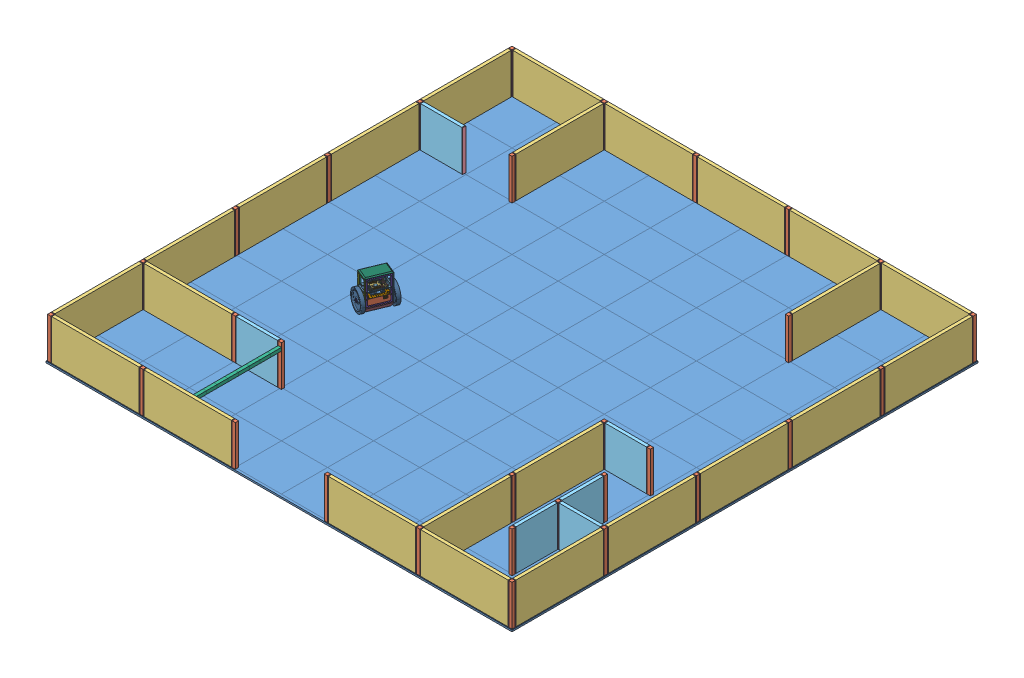
SolidWorks assembly testbed, configuration Default. Lengths in mm.
Overall size (2880 260 2880).
673 component instances, 79 part files, 153 mates.
Components (placement in the parent):
- floor-1: floor [Default] at origin size (2880 10 2880)
- post_250-1: post_250 [Default] at (-2707.5 10 -2707.5) size (20 250 20)
- post_250-2: post_250 [Default] at (-2137.5 10 -2707.5) size (20 250 20)
- post_250-3: post_250 [Default] at (-1567.5 10 -2707.5) size (20 250 20)
- post_250-4: post_250 [Default] at (-997.5 10 -2707.5) size (20 250 20)
- post_250-5: post_250 [Default] at (-427.5 10 -2707.5) size (20 250 20)
- post_250-6: post_250 [Default] at (142.5 10 -2707.5) size (20 250 20)
- post_250-7: post_250 [Default] at (-427.5 10 -2137.5) size (20 250 20)
- post_250-8: post_250 [Default] at (142.5 10 -2137.5) size (20 250 20)
- post_250-9: post_250 [Default] at (-2707.5 10 -2137.5) size (20 250 20)
- post_250-10: post_250 [Default] at (-2707.5 10 -1567.5) size (20 250 20)
- post_250-11: post_250 [Default] at (-2707.5 10 -997.5) size (20 250 20)
- post_250-12: post_250 [Default] at (-2707.5 10 -427.5) size (20 250 20)
- post_250-13: post_250 [Default] at (-2707.5 10 142.5) size (20 250 20)
- post_250-14: post_250 [Default] at (-2137.5 10 142.5) size (20 250 20)
- post_250-15: post_250 [Default] at (-2137.5 10 -427.5) size (20 250 20)
- post_250-16: post_250 [Default] at (-1567.5 10 142.5) size (20 250 20)
- post_250-17: post_250 [Default] at (-997.5 10 142.5) size (20 250 20)
- post_250-18: post_250 [Default] at (-427.5 10 142.5) size (20 250 20)
- post_250-19: post_250 [Default] at (142.5 10 142.5) size (20 250 20)
- post_250-20: post_250 [Default] at (142.5 10 -427.5) size (20 250 20)
- post_250-21: post_250 [Default] at (142.5 10 -997.5) size (20 250 20)
- post_250-22: post_250 [Default] at (142.5 10 -1567.5) size (20 250 20)
- post_250-23: post_250 [Default] at (-2137.5 10 -2137.5) size (20 250 20)
- post_250-24: post_250 [Default] at (-142.5 10 -142.5) size (20 250 20)
- post_250-25: post_250 [Default] at (-427.5 10 -427.5) size (20 250 20)
- post_250-26: post_250 [Default] at (-427.5 10 -997.5) size (20 250 20)
- post_250-27: post_250 [Default] at (-142.5 10 -427.5) size (20 250 20)
- post_250-28: post_250 [Default] at (-142.5 10 -712.5) size (20 250 20)
- post_250-29: post_250 [Default] at (-142.5 10 -997.5) size (20 250 20)
- wallelement_2-cell-1: wallelement_2-cell [Default] at (-712.5 135 132.5) size (550 250 20)
  - wall_2-cell-1: wall_2-cell [Default] at origin size (540 250 20)
  - wall_profile_hook_250-1: wall_profile_hook_250 [Default] at (275 0 10) x (0 0 1) z (-1 0 0) size (20 250 5)
  - wall_profile_hook_250-2: wall_profile_hook_250 [Default] at (-275 0 10) x (0 0 -1) z (1 0 0) size (20 250 5)
- wallelement_2-cell-2: wallelement_2-cell [Default] at (-142.5 135 132.5) size (550 250 20)
  - wall_2-cell-1: wall_2-cell [Default] at origin size (540 250 20)
  - wall_profile_hook_250-1: wall_profile_hook_250 [Default] at (275 0 10) x (0 0 1) z (-1 0 0) size (20 250 5)
  - wall_profile_hook_250-2: wall_profile_hook_250 [Default] at (-275 0 10) x (0 0 -1) z (1 0 0) size (20 250 5)
- wallelement_2-cell-3: wallelement_2-cell [Default] at (132.5 135 -142.5) x (0 0 -1) z (1 0 0) size (550 250 20)
  - wall_2-cell-1: wall_2-cell [Default] at origin size (540 250 20)
  - wall_profile_hook_250-1: wall_profile_hook_250 [Default] at (275 0 10) x (0 0 1) z (-1 0 0) size (20 250 5)
  - wall_profile_hook_250-2: wall_profile_hook_250 [Default] at (-275 0 10) x (0 0 -1) z (1 0 0) size (20 250 5)
- wallelement_2-cell-4: wallelement_2-cell [Default] at (132.5 135 -712.5) x (0 0 -1) z (1 0 0) size (550 250 20)
  - wall_2-cell-1: wall_2-cell [Default] at origin size (540 250 20)
  - wall_profile_hook_250-1: wall_profile_hook_250 [Default] at (275 0 10) x (0 0 1) z (-1 0 0) size (20 250 5)
  - wall_profile_hook_250-2: wall_profile_hook_250 [Default] at (-275 0 10) x (0 0 -1) z (1 0 0) size (20 250 5)
- wallelement_2-cell-5: wallelement_2-cell [Default] at (132.5 135 -1282.5) x (0 0 -1) z (1 0 0) size (550 250 20)
  - wall_2-cell-1: wall_2-cell [Default] at origin size (540 250 20)
  - wall_profile_hook_250-1: wall_profile_hook_250 [Default] at (275 0 10) x (0 0 1) z (-1 0 0) size (20 250 5)
  - wall_profile_hook_250-2: wall_profile_hook_250 [Default] at (-275 0 10) x (0 0 -1) z (1 0 0) size (20 250 5)
- wallelement_2-cell-6: wallelement_2-cell [Default] at (132.5 135 -1852.5) x (0 0 -1) z (1 0 0) size (550 250 20)
  - wall_2-cell-1: wall_2-cell [Default] at origin size (540 250 20)
  - wall_profile_hook_250-1: wall_profile_hook_250 [Default] at (275 0 10) x (0 0 1) z (-1 0 0) size (20 250 5)
  - wall_profile_hook_250-2: wall_profile_hook_250 [Default] at (-275 0 10) x (0 0 -1) z (1 0 0) size (20 250 5)
- wallelement_2-cell-7: wallelement_2-cell [Default] at (132.5 135 -2422.5) x (0 0 -1) z (1 0 0) size (550 250 20)
  - wall_2-cell-1: wall_2-cell [Default] at origin size (540 250 20)
  - wall_profile_hook_250-1: wall_profile_hook_250 [Default] at (275 0 10) x (0 0 1) z (-1 0 0) size (20 250 5)
  - wall_profile_hook_250-2: wall_profile_hook_250 [Default] at (-275 0 10) x (0 0 -1) z (1 0 0) size (20 250 5)
- wallelement_2-cell-8: wallelement_2-cell [Default] at (-142.5 135 -2717.5) size (550 250 20)
  - wall_2-cell-1: wall_2-cell [Default] at origin size (540 250 20)
  - wall_profile_hook_250-1: wall_profile_hook_250 [Default] at (275 0 10) x (0 0 1) z (-1 0 0) size (20 250 5)
  - wall_profile_hook_250-2: wall_profile_hook_250 [Default] at (-275 0 10) x (0 0 -1) z (1 0 0) size (20 250 5)
- wallelement_2-cell-9: wallelement_2-cell [Default] at (-712.5 135 -2717.5) size (550 250 20)
  - wall_2-cell-1: wall_2-cell [Default] at origin size (540 250 20)
  - wall_profile_hook_250-1: wall_profile_hook_250 [Default] at (275 0 10) x (0 0 1) z (-1 0 0) size (20 250 5)
  - wall_profile_hook_250-2: wall_profile_hook_250 [Default] at (-275 0 10) x (0 0 -1) z (1 0 0) size (20 250 5)
- wallelement_2-cell-10: wallelement_2-cell [Default] at (-1282.5 135 -2717.5) size (550 250 20)
  - wall_2-cell-1: wall_2-cell [Default] at origin size (540 250 20)
  - wall_profile_hook_250-1: wall_profile_hook_250 [Default] at (275 0 10) x (0 0 1) z (-1 0 0) size (20 250 5)
  - wall_profile_hook_250-2: wall_profile_hook_250 [Default] at (-275 0 10) x (0 0 -1) z (1 0 0) size (20 250 5)
- wallelement_2-cell-11: wallelement_2-cell [Default] at (-1852.5 135 -2717.5) size (550 250 20)
  - wall_2-cell-1: wall_2-cell [Default] at origin size (540 250 20)
  - wall_profile_hook_250-1: wall_profile_hook_250 [Default] at (275 0 10) x (0 0 1) z (-1 0 0) size (20 250 5)
  - wall_profile_hook_250-2: wall_profile_hook_250 [Default] at (-275 0 10) x (0 0 -1) z (1 0 0) size (20 250 5)
- wallelement_2-cell-12: wallelement_2-cell [Default] at (-2422.5 135 -2717.5) size (550 250 20)
  - wall_2-cell-1: wall_2-cell [Default] at origin size (540 250 20)
  - wall_profile_hook_250-1: wall_profile_hook_250 [Default] at (275 0 10) x (0 0 1) z (-1 0 0) size (20 250 5)
  - wall_profile_hook_250-2: wall_profile_hook_250 [Default] at (-275 0 10) x (0 0 -1) z (1 0 0) size (20 250 5)
- wallelement_2-cell-13: wallelement_2-cell [Default] at (-417.5 135 -2422.5) x (0 0 1) z (-1 0 0) size (550 250 20)
  - wall_2-cell-1: wall_2-cell [Default] at origin size (540 250 20)
  - wall_profile_hook_250-1: wall_profile_hook_250 [Default] at (275 0 10) x (0 0 1) z (-1 0 0) size (20 250 5)
  - wall_profile_hook_250-2: wall_profile_hook_250 [Default] at (-275 0 10) x (0 0 -1) z (1 0 0) size (20 250 5)
- wallelement_2-cell-14: wallelement_2-cell [Default] at (-2717.5 135 -2422.5) x (0 0 -1) z (1 0 0) size (550 250 20)
  - wall_2-cell-1: wall_2-cell [Default] at origin size (540 250 20)
  - wall_profile_hook_250-1: wall_profile_hook_250 [Default] at (275 0 10) x (0 0 1) z (-1 0 0) size (20 250 5)
  - wall_profile_hook_250-2: wall_profile_hook_250 [Default] at (-275 0 10) x (0 0 -1) z (1 0 0) size (20 250 5)
- wallelement_2-cell-15: wallelement_2-cell [Default] at (-2697.5 135 -1852.5) x (0 0 1) z (-1 0 0) size (550 250 20)
  - wall_2-cell-1: wall_2-cell [Default] at origin size (540 250 20)
  - wall_profile_hook_250-1: wall_profile_hook_250 [Default] at (275 0 10) x (0 0 1) z (-1 0 0) size (20 250 5)
  - wall_profile_hook_250-2: wall_profile_hook_250 [Default] at (-275 0 10) x (0 0 -1) z (1 0 0) size (20 250 5)
- wallelement_2-cell-16: wallelement_2-cell [Default] at (-2697.5 135 -1282.5) x (0 0 1) z (-1 0 0) size (550 250 20)
  - wall_2-cell-1: wall_2-cell [Default] at origin size (540 250 20)
  - wall_profile_hook_250-1: wall_profile_hook_250 [Default] at (275 0 10) x (0 0 1) z (-1 0 0) size (20 250 5)
  - wall_profile_hook_250-2: wall_profile_hook_250 [Default] at (-275 0 10) x (0 0 -1) z (1 0 0) size (20 250 5)
- wallelement_2-cell-17: wallelement_2-cell [Default] at (-2697.5 135 -712.5) x (0 0 1) z (-1 0 0) size (550 250 20)
  - wall_2-cell-1: wall_2-cell [Default] at origin size (540 250 20)
  - wall_profile_hook_250-1: wall_profile_hook_250 [Default] at (275 0 10) x (0 0 1) z (-1 0 0) size (20 250 5)
  - wall_profile_hook_250-2: wall_profile_hook_250 [Default] at (-275 0 10) x (0 0 -1) z (1 0 0) size (20 250 5)
- wallelement_2-cell-18: wallelement_2-cell [Default] at (-2697.5 135 -142.5) x (0 0 1) z (-1 0 0) size (550 250 20)
  - wall_2-cell-1: wall_2-cell [Default] at origin size (540 250 20)
  - wall_profile_hook_250-1: wall_profile_hook_250 [Default] at (275 0 10) x (0 0 1) z (-1 0 0) size (20 250 5)
  - wall_profile_hook_250-2: wall_profile_hook_250 [Default] at (-275 0 10) x (0 0 -1) z (1 0 0) size (20 250 5)
- wallelement_2-cell-19: wallelement_2-cell [Default] at (-2422.5 135 132.5) size (550 250 20)
  - wall_2-cell-1: wall_2-cell [Default] at origin size (540 250 20)
  - wall_profile_hook_250-1: wall_profile_hook_250 [Default] at (275 0 10) x (0 0 1) z (-1 0 0) size (20 250 5)
  - wall_profile_hook_250-2: wall_profile_hook_250 [Default] at (-275 0 10) x (0 0 -1) z (1 0 0) size (20 250 5)
- wallelement_2-cell-20: wallelement_2-cell [Default] at (-1852.5 135 132.5) size (550 250 20)
  - wall_2-cell-1: wall_2-cell [Default] at origin size (540 250 20)
  - wall_profile_hook_250-1: wall_profile_hook_250 [Default] at (275 0 10) x (0 0 1) z (-1 0 0) size (20 250 5)
  - wall_profile_hook_250-2: wall_profile_hook_250 [Default] at (-275 0 10) x (0 0 -1) z (1 0 0) size (20 250 5)
- wallelement_2-cell-21: wallelement_2-cell [Default] at (-2422.5 135 -437.5) size (550 250 20)
  - wall_2-cell-1: wall_2-cell [Default] at origin size (540 250 20)
  - wall_profile_hook_250-1: wall_profile_hook_250 [Default] at (275 0 10) x (0 0 1) z (-1 0 0) size (20 250 5)
  - wall_profile_hook_250-2: wall_profile_hook_250 [Default] at (-275 0 10) x (0 0 -1) z (1 0 0) size (20 250 5)
- wallelement_2-cell-22: wallelement_2-cell [Default] at (-437.5 135 -142.5) x (0 0 -1) z (1 0 0) size (550 250 20)
  - wall_2-cell-1: wall_2-cell [Default] at origin size (540 250 20)
  - wall_profile_hook_250-1: wall_profile_hook_250 [Default] at (275 0 10) x (0 0 1) z (-1 0 0) size (20 250 5)
  - wall_profile_hook_250-2: wall_profile_hook_250 [Default] at (-275 0 10) x (0 0 -1) z (1 0 0) size (20 250 5)
- wallelement_2-cell-23: wallelement_2-cell [Default] at (-437.5 135 -712.5) x (0 0 -1) z (1 0 0) size (550 250 20)
  - wall_2-cell-1: wall_2-cell [Default] at origin size (540 250 20)
  - wall_profile_hook_250-1: wall_profile_hook_250 [Default] at (275 0 10) x (0 0 1) z (-1 0 0) size (20 250 5)
  - wall_profile_hook_250-2: wall_profile_hook_250 [Default] at (-275 0 10) x (0 0 -1) z (1 0 0) size (20 250 5)
- wallelement_2-cell-24: wallelement_2-cell [Default] at (-2147.5 135 -2422.5) x (0 0 -1) z (1 0 0) size (550 250 20)
  - wall_2-cell-1: wall_2-cell [Default] at origin size (540 250 20)
  - wall_profile_hook_250-1: wall_profile_hook_250 [Default] at (275 0 10) x (0 0 1) z (-1 0 0) size (20 250 5)
  - wall_profile_hook_250-2: wall_profile_hook_250 [Default] at (-275 0 10) x (0 0 -1) z (1 0 0) size (20 250 5)
- twipr-1: twipr [Default] at (-1820.3783 -75.269 -1556.7406) x (0.381849 0 -0.924225) z (0.924225 0 0.381849) size (189.01 198.92 123.83)
  - twipr_sketch-1: twipr_sketch [Default] at origin (hidden)
  - brace_left-1: brace_left [Default] at (-379.6774 202.2203 0) x (0 0 -1) z (1 0 0) size (80 150 10.2)
  - brace_front-1: brace_front [Default] at (-442.6774 202.2203 -40) size (126 150 7)
  - brace_right-1: brace_right [Default] at (-505.6774 202.2203 0) x (0 0 1) z (-1 0 0) size (80 150 7)
  - brace_back-1: brace_back [Default] at (-442.6774 202.2203 33) size (126 150 7)
  - platform_middle-1: platform_middle [Default] at (-442.7274 165.7203 0) size (126 42 78)
  - banebots_4_78-1: banebots_4_78 [Default] at (-368.872 147.2203 0) x (0 0 -1) z (1 0 0) size (123.83 123.83 21.34)
  - banebots_4_78-2: banebots_4_78 [Default] at (-516.2261 147.2203 0) x (0 0 1) z (-1 0 0) size (123.83 123.83 21.34)
  - robot-hub-1: robot-hub [Default] at (-323.8774 211.7203 115.5) x (-1 0 0) z (0 1 0) size (91.46 70 13.31)
    - robot-hub.step-1: robot-hub.step [Default] at origin size (91.46 70 13.31)
      - R_0603_1608Metric.step-1: R_0603_1608Metric.step [Default] at (112.6 -91.1 1.71) x (0 1 0) z (0 0 1) size (1.6 0.8 0.45)
        - SOLID.step-1: SOLID.step [Default] at origin size (1.6 0.8 0.45)
      - C_1210_3225Metric.step-1: C_1210_3225Metric.step [Default] at (76.55 -102.85 1.71) x (-1 0 0) z (0 0 1) size (3.2 2.5 2.5)
        - SOLID-0.step-1: SOLID-0.step [Default] at origin size (3.2 2.5 2.5)
      - C_0603_1608Metric.step-1: C_0603_1608Metric.step [Default] at (132.2 -95.8 1.71) x (0 1 0) z (0 0 1) size (1.6 0.8 0.8)
        - SOLID-1.step-1: SOLID-1.step [Default] at origin size (1.6 0.8 0.8)
      - JST_GH_BM04B-GHS-TBT_1x04-1MP_P1.25mm_Vertical.step-1: JST_GH_BM04B-GHS-TBT_1x04-1MP_P1.25mm_Vertical.step [Default] at (152.6 -95.3 1.71) x (0 1 0) z (0 0 1) size (8.25 4.95 4.2)
        - SOLID-2.step-1: SOLID-2.step [Default] at origin size (8.25 4.95 4.2)
      - R_0603_1608Metric.step-2: R_0603_1608Metric.step [Default] at (107.5 -84.7687 1.71) x (0 -1 0) z (0 0 1) size (1.6 0.8 0.45)
        - SOLID.step-1: SOLID.step [Default] at origin size (1.6 0.8 0.45)
      - R_0402_1005Metric.step-1: R_0402_1005Metric.step [Default] at (123.5 -93.2 1.71) x (0 1 0) z (0 0 1) size (1 0.5 0.35)
        - SOLID-3.step-1: SOLID-3.step [Default] at origin size (1 0.5 0.35)
      - LED_0603_1608Metric.step-1: LED_0603_1608Metric.step [Default] at (88 -81.3 1.71) x (0 -1 0) z (0 0 1) size (1.6 0.8 1.1)
        - SOLID-4.step-1: SOLID-4.step [Default] at origin size (1.6 0.8 1.1)
      - R_0603_1608Metric.step-3: R_0603_1608Metric.step [Default] at (113.4 -101.6 1.71) x (-1 0 0) z (0 0 1) size (1.6 0.8 0.45)
        - SOLID.step-1: SOLID.step [Default] at origin size (1.6 0.8 0.45)
      - LTC4412ES6#TRMPBF.step-1: LTC4412ES6#TRMPBF.step [Default] at (86.1 -94.6 1.71) size (2.8 2.9 1)
        - COMPOUND.step-1: COMPOUND.step [Default] at origin size (2.8 2.9 1)
      - ws2812_2020.step-1: ws2812_2020.step [Default] at (84.3 -81.3 1.71) size (2.2 2 0.84)
        - COMPOUND-5.step-1: COMPOUND-5.step [Default] at origin size (2.2 2 0.84)
      - LED_0603_1608Metric.step-2: LED_0603_1608Metric.step [Default] at (86.1 -86.8 1.71) size (1.6 0.8 1.1)
        - SOLID-4.step-1: SOLID-4.step [Default] at origin size (1.6 0.8 1.1)
      - R_0402_1005Metric.step-2: R_0402_1005Metric.step [Default] at (133.8 -92.9 1.71) x (0 -1 0) z (0 0 1) size (1 0.5 0.35)
        - SOLID-3.step-1: SOLID-3.step [Default] at origin size (1 0.5 0.35)
      - JST_GH_BM06B-GHS-TBT_1x06-1MP_P1.25mm_Vertical.step-1: JST_GH_BM06B-GHS-TBT_1x06-1MP_P1.25mm_Vertical.step [Default] at (114 -135.2 1.71) size (10.75 4.95 4.2)
        - SOLID-6.step-1: SOLID-6.step [Default] at origin size (10.75 4.95 4.2)
      - JST_GH_BM04B-GHS-TBT_1x04-1MP_P1.25mm_Vertical.step-2: JST_GH_BM04B-GHS-TBT_1x04-1MP_P1.25mm_Vertical.step [Default] at (134.6 -135.2 1.71) size (8.25 4.95 4.2)
        - SOLID-2.step-1: SOLID-2.step [Default] at origin size (8.25 4.95 4.2)
      - C_0603_1608Metric.step-2: C_0603_1608Metric.step [Default] at (109.4 -97.4 1.71) x (-1 0 0) z (0 0 1) size (1.6 0.8 0.8)
        - SOLID-1.step-1: SOLID-1.step [Default] at origin size (1.6 0.8 0.8)
      - C_1210_3225Metric.step-2: C_1210_3225Metric.step [Default] at (87.55 -126.8 1.71) size (3.2 2.5 2.5)
        - SOLID-0.step-1: SOLID-0.step [Default] at origin size (3.2 2.5 2.5)
      - C_1210_3225Metric.step-3: C_1210_3225Metric.step [Default] at (76.55 -109.6 1.71) x (-1 0 0) z (0 0 1) size (3.2 2.5 2.5)
        - SOLID-0.step-1: SOLID-0.step [Default] at origin size (3.2 2.5 2.5)
      - R_0603_1608Metric.step-4: R_0603_1608Metric.step [Default] at (138.6 -95.5 1.71) x (0 -1 0) z (0 0 1) size (1.6 0.8 0.45)
        - SOLID.step-1: SOLID.step [Default] at origin size (1.6 0.8 0.45)
      - CP_Elec_6.3x5.2.step-1: CP_Elec_6.3x5.2.step [Default] at (77.8 -133.7 1.71) x (0 1 0) z (0 0 1) size (10.2 10.92 5.2)
        - SOLID-7.step-1: SOLID-7.step [Default] at origin size (10.2 10.92 5.2)
      - R_0402_1005Metric.step-3: R_0402_1005Metric.step [Default] at (127.9 -91.7 1.71) x (0 -1 0) z (0 0 1) size (1 0.5 0.35)
        - SOLID-3.step-1: SOLID-3.step [Default] at origin size (1 0.5 0.35)
      - R_0603_1608Metric.step-5: R_0603_1608Metric.step [Default] at (104.2 -119.8 1.71) size (1.6 0.8 0.45)
        - SOLID.step-1: SOLID.step [Default] at origin size (1.6 0.8 0.45)
      - C_0603_1608Metric.step-3: C_0603_1608Metric.step [Default] at (132 -113.2 1.71) x (0 -1 0) z (0 0 1) size (1.6 0.8 0.8)
        - SOLID-1.step-1: SOLID-1.step [Default] at origin size (1.6 0.8 0.8)
      - JST_GH_BM04B-GHS-TBT_1x04-1MP_P1.25mm_Vertical.step-3: JST_GH_BM04B-GHS-TBT_1x04-1MP_P1.25mm_Vertical.step [Default] at (97.4 -125.1 1.71) size (8.25 4.95 4.2)
        - SOLID-2.step-1: SOLID-2.step [Default] at origin size (8.25 4.95 4.2)
      - C_0603_1608Metric.step-4: C_0603_1608Metric.step [Default] at (87.8 -117.65 1.71) x (0 -1 0) z (0 0 1) size (1.6 0.8 0.8)
        - SOLID-1.step-1: SOLID-1.step [Default] at origin size (1.6 0.8 0.8)
      - JST_GH_BM06B-GHS-TBT_1x06-1MP_P1.25mm_Vertical.step-2: JST_GH_BM06B-GHS-TBT_1x06-1MP_P1.25mm_Vertical.step [Default] at (160.6 -106.3 1.71) x (0 1 0) z (0 0 1) size (10.75 4.95 4.2)
        - SOLID-6.step-1: SOLID-6.step [Default] at origin size (10.75 4.95 4.2)
      - JST_GH_BM02B-GHS-TBT_1x02-1MP_P1.25mm_Vertical.step-1: JST_GH_BM02B-GHS-TBT_1x02-1MP_P1.25mm_Vertical.step [Default] at (152.5 -143.25 1.71) size (5.75 4.95 4.2)
        - SOLID-8.step-1: SOLID-8.step [Default] at origin size (5.75 4.95 4.2)
      - USB4105-GF-A.step-1: USB4105-GF-A.step [Default] at (76.635 -88.9375 1.71) x (0 -1 0) z (-1 0 0) size (9.58 4.16 7.71)
        - COMPOUND-9.step-1: COMPOUND-9.step [Default] at origin size (9.58 4.16 7.71)
      - JST_GH_BM04B-GHS-TBT_1x04-1MP_P1.25mm_Vertical.step-4: JST_GH_BM04B-GHS-TBT_1x04-1MP_P1.25mm_Vertical.step [Default] at (160.6 -95.3 1.71) x (0 1 0) z (0 0 1) size (8.25 4.95 4.2)
        - SOLID-2.step-1: SOLID-2.step [Default] at origin size (8.25 4.95 4.2)
      - 4341x30258x6 (rev1).step-1: 4341x30258x6 (rev1).step [Default] at (104.2 -116 1.71) x (1 0 0) z (0 -1 0) size (3.2 2.5 4.6)
        - COMPOUND-10.step-1: COMPOUND-10.step [Default] at origin size (3.2 2.5 4.6)
      - JST_GH_BM04B-GHS-TBT_1x04-1MP_P1.25mm_Vertical.step-5: JST_GH_BM04B-GHS-TBT_1x04-1MP_P1.25mm_Vertical.step [Default] at (103.2 -143.2 1.71) size (8.25 4.95 4.2)
        - SOLID-2.step-1: SOLID-2.step [Default] at origin size (8.25 4.95 4.2)
      - C_0805_2012Metric.step-1: C_0805_2012Metric.step [Default] at (112.7 -112 1.71) x (0 1 0) z (0 0 1) size (2 1.25 1.25)
        - SOLID-11.step-1: SOLID-11.step [Default] at origin size (2 1.25 1.25)
      - CUI_DEVICES_CMT-7525-80-SMT-TR.step-1: CUI_DEVICES_CMT-7525-80-SMT-TR.step [Default] at (97.3 -115.8 1.71) x (1 0 0) z (0 -1 0) size (7.5 2.5 7.5)
        - COMPOUND-12.step-1: COMPOUND-12.step [Default] at origin size (7.5 2.5 7.5)
      - BMX160.step-1: BMX160.step [Default] at (111.35 -94.75 1.71) x (0 -1 0) z (-1 0 0) size (3 1 2.5)
        - COMPOUND-13.step-1: COMPOUND-13.step [Default] at origin size (3 1 2.5)
      - PinHeader_2x15_P2.54mm_Vertical.step-1: PinHeader_2x15_P2.54mm_Vertical.step [Default] at (110.525 -127.545 1.71) x (0 1 0) z (0 0 1) size (5.08 38.1 11.54)
        - SOLID-14.step-1: SOLID-14.step [Default] at origin size (5.08 38.1 11.54)
      - C_0603_1608Metric.step-5: C_0603_1608Metric.step [Default] at (115.5 -93.3 1.71) x (0 1 0) z (0 0 1) size (1.6 0.8 0.8)
        - SOLID-1.step-1: SOLID-1.step [Default] at origin size (1.6 0.8 0.8)
      - JST_GH_BM02B-GHS-TBT_1x02-1MP_P1.25mm_Vertical.step-2: JST_GH_BM02B-GHS-TBT_1x02-1MP_P1.25mm_Vertical.step [Default] at (152.5 -135.25 1.71) size (5.75 4.95 4.2)
        - SOLID-8.step-1: SOLID-8.step [Default] at origin size (5.75 4.95 4.2)
      - FTSH-105-01-L-DV-K.step-1: FTSH-105-01-L-DV-K.step [Default] at (97.4 -106.5 2.21) x (-1 0 0) z (0 1 0) size (6.35 6.12 5.84)
        - COMPOUND-15.step-1: COMPOUND-15.step [Default] at origin size (6.35 6.12 5.84)
      - JST_GH_BM04B-GHS-TBT_1x04-1MP_P1.25mm_Vertical.step-6: JST_GH_BM04B-GHS-TBT_1x04-1MP_P1.25mm_Vertical.step [Default] at (103.2 -135.2 1.71) size (8.25 4.95 4.2)
        - SOLID-2.step-1: SOLID-2.step [Default] at origin size (8.25 4.95 4.2)
      - C_0603_1608Metric.step-6: C_0603_1608Metric.step [Default] at (141.5 -98.8 1.71) x (0 1 0) z (0 0 1) size (1.6 0.8 0.8)
        - SOLID-1.step-1: SOLID-1.step [Default] at origin size (1.6 0.8 0.8)
      - ECS-250-18-33B-CKY-TR.step-1: ECS-250-18-33B-CKY-TR.step [Default] at (140.9 -104.6 1.71) x (0 1 0) z (0 0 1) size (3.38 2.78 0.9)
        - COMPOUND-16.step-1: COMPOUND-16.step [Default] at origin size (3.38 2.78 0.9)
      - C_0603_1608Metric.step-7: C_0603_1608Metric.step [Default] at (114.5 -112.3 1.71) x (0 1 0) z (0 0 1) size (1.6 0.8 0.8)
        - SOLID-1.step-1: SOLID-1.step [Default] at origin size (1.6 0.8 0.8)
      - JST_GH_BM06B-GHS-TBT_1x06-1MP_P1.25mm_Vertical.step-3: JST_GH_BM06B-GHS-TBT_1x06-1MP_P1.25mm_Vertical.step [Default] at (113.95 -143.2 1.71) size (10.75 4.95 4.2)
        - SOLID-6.step-1: SOLID-6.step [Default] at origin size (10.75 4.95 4.2)
      - C_0603_1608Metric.step-8: C_0603_1608Metric.step [Default] at (134.9 -106.6 1.71) x (0 -1 0) z (0 0 1) size (1.6 0.8 0.8)
        - SOLID-1.step-1: SOLID-1.step [Default] at origin size (1.6 0.8 0.8)
      - SOT-323_SC-70.step-1: SOT-323_SC-70.step [Default] at (140.9 -95.4 1.71) x (0 1 0) z (0 0 1) size (2 2 1.05)
        - SOLID-17.step-1: SOLID-17.step [Default] at origin size (2 2 1.05)
      - LED_0603_1608Metric.step-3: LED_0603_1608Metric.step [Default] at (109.4 -100.1 1.71) x (0 -1 0) z (0 0 1) size (1.6 0.8 1.1)
        - SOLID-4.step-1: SOLID-4.step [Default] at origin size (1.6 0.8 1.1)
      - LMR33630ADDA.step-1: LMR33630ADDA.step [Default] at (84.05 -119.1 1.71) x (0 1 0) z (0 0 1) size (6 4.9 1.7)
        - COMPOUND-18.step-1: COMPOUND-18.step [Default] at origin size (6 4.9 1.7)
      - C_0603_1608Metric.step-9: C_0603_1608Metric.step [Default] at (88.3 -124.4 1.71) size (1.6 0.8 0.8)
        - SOLID-1.step-1: SOLID-1.step [Default] at origin size (1.6 0.8 0.8)
      - C_0603_1608Metric.step-10: C_0603_1608Metric.step [Default] at (140.8 -101.1 1.71) size (1.6 0.8 0.8)
        - SOLID-1.step-1: SOLID-1.step [Default] at origin size (1.6 0.8 0.8)
      - PinHeader_2x04_P2.00mm_Vertical.step-1: PinHeader_2x04_P2.00mm_Vertical.step [Default] at (149.4 -81.4 1.71) x (0 1 0) z (0 0 1) size (4 8 8.8)
        - SOLID-19.step-1: SOLID-19.step [Default] at origin size (4 8 8.8)
      - 1-1734248-5.step-1: 1-1734248-5.step [Default] at (159.98 -126.3 6.21) x (0 1 0) z (0 0 1) size (22.4 4.85 5.68)
        - SOLID-20.step-1: SOLID-20.step [Default] at origin size (22.4 4.85 5.68)
      - IS25LP032D-JNLA3-TR.step-1: IS25LP032D-JNLA3-TR.step [Default] at (84.9 -99.3 1.71) x (-1 0 0) z (0 0 1) size (6 4.9 1.75)
        - COMPOUND-21.step-1: COMPOUND-21.step [Default] at origin size (6 4.9 1.75)
      - 691313510002.step-1: 691313510002.step [Default] at (89.3 -135.2 5.71) x (-1 0 0) z (0 -1 0) size (12.16 12 12)
        - COMPOUND-22.step-1: COMPOUND-22.step [Default] at origin size (12.16 12 12)
      - LED_0603_1608Metric.step-4: LED_0603_1608Metric.step [Default] at (93 -81.3 1.71) x (0 -1 0) z (0 0 1) size (1.6 0.8 1.1)
        - SOLID-4.step-1: SOLID-4.step [Default] at origin size (1.6 0.8 1.1)
      - JST_GH_BM04B-GHS-TBT_1x04-1MP_P1.25mm_Vertical.step-7: JST_GH_BM04B-GHS-TBT_1x04-1MP_P1.25mm_Vertical.step [Default] at (124.95 -135.2 1.71) size (8.25 4.95 4.2)
        - SOLID-2.step-1: SOLID-2.step [Default] at origin size (8.25 4.95 4.2)
      - LED_0603_1608Metric.step-5: LED_0603_1608Metric.step [Default] at (154.5 -117.4 1.71) x (0 -1 0) z (0 0 1) size (1.6 0.8 1.1)
        - SOLID-4.step-1: SOLID-4.step [Default] at origin size (1.6 0.8 1.1)
      - JST_GH_BM03B-GHS-TBT_1x03-1MP_P1.25mm_Vertical.step-1: JST_GH_BM03B-GHS-TBT_1x03-1MP_P1.25mm_Vertical.step [Default] at (97.4 -98.7 1.71) size (7 4.95 4.2)
        - SOLID-23.step-1: SOLID-23.step [Default] at origin size (7 4.95 4.2)
      - C_0603_1608Metric.step-11: C_0603_1608Metric.step [Default] at (108.6 -94.8 1.71) x (0 -1 0) z (0 0 1) size (1.6 0.8 0.8)
        - SOLID-1.step-1: SOLID-1.step [Default] at origin size (1.6 0.8 0.8)
      - R_0603_1608Metric.step-6: R_0603_1608Metric.step [Default] at (113.4 -103.2 1.71) size (1.6 0.8 0.45)
        - SOLID.step-1: SOLID.step [Default] at origin size (1.6 0.8 0.45)
      - LED_0603_1608Metric.step-6: LED_0603_1608Metric.step [Default] at (95.5 -81.3 1.71) x (0 -1 0) z (0 0 1) size (1.6 0.8 1.1)
        - SOLID-4.step-1: SOLID-4.step [Default] at origin size (1.6 0.8 1.1)
      - R_0402_1005Metric.step-4: R_0402_1005Metric.step [Default] at (125.7 -93.2 1.71) x (0 -1 0) z (0 0 1) size (1 0.5 0.35)
        - SOLID-3.step-1: SOLID-3.step [Default] at origin size (1 0.5 0.35)
      - SOT-23-6.step-1: SOT-23-6.step [Default] at (86.1 -89.45 1.71) x (-1 0 0) z (0 0 1) size (2.8 2.9 1.55)
        - SOLID-24.step-1: SOLID-24.step [Default] at origin size (2.8 2.9 1.55)
      - R_0603_1608Metric.step-7: R_0603_1608Metric.step [Default] at (89.3 -117.65 1.71) x (0 -1 0) z (0 0 1) size (1.6 0.8 0.45)
        - SOLID.step-1: SOLID.step [Default] at origin size (1.6 0.8 0.45)
      - R_0603_1608Metric.step-8: R_0603_1608Metric.step [Default] at (92.3 -111.9 1.71) x (0 1 0) z (0 0 1) size (1.6 0.8 0.45)
        - SOLID.step-1: SOLID.step [Default] at origin size (1.6 0.8 0.45)
      - R_0603_1608Metric.step-9: R_0603_1608Metric.step [Default] at (88.55 -115.4 1.71) size (1.6 0.8 0.45)
        - SOLID.step-1: SOLID.step [Default] at origin size (1.6 0.8 0.45)
      - 691322110002.step-1: 691322110002.step [Default] at (101.9 -81.4 5.21) x (-1 0 0) z (0 1 0) size (8.4 10.7 9.2)
        - COMPOUND-25.step-1: COMPOUND-25.step [Default] at origin size (8.4 10.7 9.2)
      - LED_0603_1608Metric.step-7: LED_0603_1608Metric.step [Default] at (90.5 -81.3 1.71) x (0 -1 0) z (0 0 1) size (1.6 0.8 1.1)
        - SOLID-4.step-1: SOLID-4.step [Default] at origin size (1.6 0.8 1.1)
      - JST_GH_BM06B-GHS-TBT_1x06-1MP_P1.25mm_Vertical.step-4: JST_GH_BM06B-GHS-TBT_1x06-1MP_P1.25mm_Vertical.step [Default] at (152.6 -106.3 1.71) x (0 1 0) z (0 0 1) size (10.75 4.95 4.2)
        - SOLID-6.step-1: SOLID-6.step [Default] at origin size (10.75 4.95 4.2)
      - R_0603_1608Metric.step-10: R_0603_1608Metric.step [Default] at (140 -98.8 1.71) x (0 -1 0) z (0 0 1) size (1.6 0.8 0.45)
        - SOLID.step-1: SOLID.step [Default] at origin size (1.6 0.8 0.45)
      - C_1210_3225Metric.step-4: C_1210_3225Metric.step [Default] at (79.6 -126.9 1.71) x (-1 0 0) z (0 0 1) size (3.2 2.5 2.5)
        - SOLID-0.step-1: SOLID-0.step [Default] at origin size (3.2 2.5 2.5)
      - JST_GH_BM04B-GHS-TBT_1x04-1MP_P1.25mm_Vertical.step-8: JST_GH_BM04B-GHS-TBT_1x04-1MP_P1.25mm_Vertical.step [Default] at (134.6 -143.2 1.71) size (8.25 4.95 4.2)
        - SOLID-2.step-1: SOLID-2.step [Default] at origin size (8.25 4.95 4.2)
      - PDS760-13.step-1: PDS760-13.step [Default] at (77.99 -118.49 1.71) x (1 0 0) z (0 -1 0) size (3.9 1.05 6.4)
        - COMPOUND-26.step-1: COMPOUND-26.step [Default] at origin size (3.9 1.05 6.4)
      - PinHeader_2x15_P2.54mm_Vertical.step-2: PinHeader_2x15_P2.54mm_Vertical.step [Default] at (110.525 -81.825 1.71) x (0 1 0) z (0 0 1) size (5.08 38.1 11.54)
        - SOLID-14.step-1: SOLID-14.step [Default] at origin size (5.08 38.1 11.54)
      - LED_0603_1608Metric.step-8: LED_0603_1608Metric.step [Default] at (96.8 -143.9 1.71) x (0 -1 0) z (0 0 1) size (1.6 0.8 1.1)
        - SOLID-4.step-1: SOLID-4.step [Default] at origin size (1.6 0.8 1.1)
      - 744325.step-1: 744325.step [Default] at (84.55 -108.35 1.71) x (-1 0 0) z (0 0 1) size (10.74 11.01 5.01)
        - COMPOUND-27.step-1: COMPOUND-27.step [Default] at origin size (10.74 11.01 5.01)
      - R_0603_1608Metric.step-11: R_0603_1608Metric.step [Default] at (111.05 -91.05 1.71) x (0 1 0) z (0 0 1) size (1.6 0.8 0.45)
        - SOLID.step-1: SOLID.step [Default] at origin size (1.6 0.8 0.45)
      - C_0603_1608Metric.step-12: C_0603_1608Metric.step [Default] at (140.75 -108.7 1.71) x (-1 0 0) z (0 0 1) size (1.6 0.8 0.8)
        - SOLID-1.step-1: SOLID-1.step [Default] at origin size (1.6 0.8 0.8)
      - C_0603_1608Metric.step-13: C_0603_1608Metric.step [Default] at (135.6 -109.2 1.71) size (1.6 0.8 0.8)
        - SOLID-1.step-1: SOLID-1.step [Default] at origin size (1.6 0.8 0.8)
      - R_0603_1608Metric.step-12: R_0603_1608Metric.step [Default] at (140.7 -111 1.71) size (1.6 0.8 0.45)
        - SOLID.step-1: SOLID.step [Default] at origin size (1.6 0.8 0.45)
      - LQFP-100_14x14mm_P0.5mm.step-1: LQFP-100_14x14mm_P0.5mm.step [Default] at (124 -104.2 1.71) x (-1 0 0) z (0 0 1) size (16 16 1.5)
        - SOLID-28.step-1: SOLID-28.step [Default] at origin size (16 16 1.5)
      - R_0603_1608Metric.step-13: R_0603_1608Metric.step [Default] at (87.8 -120.65 1.71) x (0 1 0) z (0 0 1) size (1.6 0.8 0.45)
        - SOLID.step-1: SOLID.step [Default] at origin size (1.6 0.8 0.45)
      - C_1210_3225Metric.step-5: C_1210_3225Metric.step [Default] at (76.55 -112.85 1.71) x (-1 0 0) z (0 0 1) size (3.2 2.5 2.5)
        - SOLID-0.step-1: SOLID-0.step [Default] at origin size (3.2 2.5 2.5)
      - R_0402_1005Metric.step-5: R_0402_1005Metric.step [Default] at (124.6 -93.2 1.71) x (0 1 0) z (0 0 1) size (1 0.5 0.35)
        - SOLID-3.step-1: SOLID-3.step [Default] at origin size (1 0.5 0.35)
      - SOT-563.step-1: SOT-563.step [Default] at (94.4 -93.9 1.71) x (0 -1 0) z (0 0 1) size (1.6 1.6 0.63)
        - SOLID-29.step-1: SOLID-29.step [Default] at origin size (1.6 1.6 0.63)
      - JST_GH_BM04B-GHS-TBT_1x04-1MP_P1.25mm_Vertical.step-9: JST_GH_BM04B-GHS-TBT_1x04-1MP_P1.25mm_Vertical.step [Default] at (144.225 -143.2344 1.71) size (8.25 4.95 4.2)
        - SOLID-2.step-1: SOLID-2.step [Default] at origin size (8.25 4.95 4.2)
      - C_1210_3225Metric.step-6: C_1210_3225Metric.step [Default] at (76.55 -106.35 1.71) x (-1 0 0) z (0 0 1) size (3.2 2.5 2.5)
        - SOLID-0.step-1: SOLID-0.step [Default] at origin size (3.2 2.5 2.5)
      - C_0603_1608Metric.step-14: C_0603_1608Metric.step [Default] at (79.8 -123.6 1.71) x (-1 0 0) z (0 0 1) size (1.6 0.8 0.8)
        - SOLID-1.step-1: SOLID-1.step [Default] at origin size (1.6 0.8 0.8)
      - R_0402_1005Metric.step-6: R_0402_1005Metric.step [Default] at (129 -91.7 1.71) x (0 -1 0) z (0 0 1) size (1 0.5 0.35)
        - SOLID-3.step-1: SOLID-3.step [Default] at origin size (1 0.5 0.35)
      - LED_0603_1608Metric.step-9: LED_0603_1608Metric.step [Default] at (107.5 -81.6688 1.71) x (0 -1 0) z (0 0 1) size (1.6 0.8 1.1)
        - SOLID-4.step-1: SOLID-4.step [Default] at origin size (1.6 0.8 1.1)
      - JST_GH_BM04B-GHS-TBT_1x04-1MP_P1.25mm_Vertical.step-10: JST_GH_BM04B-GHS-TBT_1x04-1MP_P1.25mm_Vertical.step [Default] at (124.95 -143.2 1.71) size (8.25 4.95 4.2)
        - SOLID-2.step-1: SOLID-2.step [Default] at origin size (8.25 4.95 4.2)
      - LED_0603_1608Metric.step-10: LED_0603_1608Metric.step [Default] at (152.6 -117.4 1.71) x (0 -1 0) z (0 0 1) size (1.6 0.8 1.1)
        - SOLID-4.step-1: SOLID-4.step [Default] at origin size (1.6 0.8 1.1)
      - C_0805_2012Metric.step-2: C_0805_2012Metric.step [Default] at (117.4 -93.1 1.71) x (0 -1 0) z (0 0 1) size (2 1.25 1.25)
        - SOLID-11.step-1: SOLID-11.step [Default] at origin size (2 1.25 1.25)
      - C_0603_1608Metric.step-15: C_0603_1608Metric.step [Default] at (135 -100.5 1.71) x (0 -1 0) z (0 0 1) size (1.6 0.8 0.8)
        - SOLID-1.step-1: SOLID-1.step [Default] at origin size (1.6 0.8 0.8)
      - R_0603_1608Metric.step-14: R_0603_1608Metric.step [Default] at (89 -94.6 1.71) x (0 -1 0) z (0 0 1) size (1.6 0.8 0.45)
        - SOLID.step-1: SOLID.step [Default] at origin size (1.6 0.8 0.45)
      - JST_GH_BM04B-GHS-TBT_1x04-1MP_P1.25mm_Vertical.step-11: JST_GH_BM04B-GHS-TBT_1x04-1MP_P1.25mm_Vertical.step [Default] at (144.225 -135.2344 1.71) size (8.25 4.95 4.2)
        - SOLID-2.step-1: SOLID-2.step [Default] at origin size (8.25 4.95 4.2)
      - R_0603_1608Metric.step-15: R_0603_1608Metric.step [Default] at (99.6 -129.6 -0.05) x (0 1 0) z (0 0 -1) size (1.6 0.8 0.45)
        - SOLID.step-1: SOLID.step [Default] at origin size (1.6 0.8 0.45)
      - C_0603_1608Metric.step-16: C_0603_1608Metric.step [Default] at (131.9625 -133.35 -0.05) x (0 1 0) z (0 0 -1) size (1.6 0.8 0.8)
        - SOLID-1.step-1: SOLID-1.step [Default] at origin size (1.6 0.8 0.8)
      - R_0603_1608Metric.step-16: R_0603_1608Metric.step [Default] at (119.6 -120.9 -0.05) x (-1 0 0) z (0 0 -1) size (1.6 0.8 0.45)
        - SOLID.step-1: SOLID.step [Default] at origin size (1.6 0.8 0.45)
      - R_0402_1005Metric.step-7: R_0402_1005Metric.step [Default] at (97.7 -85.3 -0.05) x (0 1 0) z (0 0 -1) size (1 0.5 0.35)
        - SOLID-3.step-1: SOLID-3.step [Default] at origin size (1 0.5 0.35)
      - C_0805_2012Metric.step-3: C_0805_2012Metric.step [Default] at (92.5 -98.9 -0.05) x (0 -1 0) z (0 0 -1) size (2 1.25 1.25)
        - SOLID-11.step-1: SOLID-11.step [Default] at origin size (2 1.25 1.25)
      - R_0402_1005Metric.step-8: R_0402_1005Metric.step [Default] at (91.95 -90.35 -0.05) x (-1 0 0) z (0 0 -1) size (1 0.5 0.35)
        - SOLID-3.step-1: SOLID-3.step [Default] at origin size (1 0.5 0.35)
      - MSOP-10_3x3mm_P0.5mm.step-1: MSOP-10_3x3mm_P0.5mm.step [Default] at (111.8 -114.8 -0.05) x (-1 0 0) z (0 0 -1) size (4.9 3 0.95)
        - SOLID-30.step-1: SOLID-30.step [Default] at origin size (4.9 3 0.95)
      - STM32G031G6U6.step-1: STM32G031G6U6.step [Default] at (95.6 -89.05 -0.05) x (0 1 0) z (0 0 -1) size (4.1 4.1 0.6)
        - COMPOUND-31.step-1: COMPOUND-31.step [Default] at origin size (4.1 4.1 0.6)
      - R_0603_1608Metric.step-17: R_0603_1608Metric.step [Default] at (137.5 -144 -0.05) x (0 -1 0) z (0 0 -1) size (1.6 0.8 0.45)
        - SOLID.step-1: SOLID.step [Default] at origin size (1.6 0.8 0.45)
      - R_0603_1608Metric.step-18: R_0603_1608Metric.step [Default] at (137.4625 -136.35 -0.05) x (0 -1 0) z (0 0 -1) size (1.6 0.8 0.45)
        - SOLID.step-1: SOLID.step [Default] at origin size (1.6 0.8 0.45)
      - C_0603_1608Metric.step-17: C_0603_1608Metric.step [Default] at (139 -140.9 -0.05) x (0 1 0) z (0 0 -1) size (1.6 0.8 0.8)
        - SOLID-1.step-1: SOLID-1.step [Default] at origin size (1.6 0.8 0.8)
      - R_0603_1608Metric.step-19: R_0603_1608Metric.step [Default] at (97.5 -137.2 -0.05) x (0 1 0) z (0 0 -1) size (1.6 0.8 0.45)
        - SOLID.step-1: SOLID.step [Default] at origin size (1.6 0.8 0.45)
      - R_0603_1608Metric.step-20: R_0603_1608Metric.step [Default] at (117.6 -113.8 -0.05) x (-1 0 0) z (0 0 -1) size (1.6 0.8 0.45)
        - SOLID.step-1: SOLID.step [Default] at origin size (1.6 0.8 0.45)
      - R_0603_1608Metric.step-21: R_0603_1608Metric.step [Default] at (156.7 -115 -0.05) x (0 1 0) z (0 0 -1) size (1.6 0.8 0.45)
        - SOLID.step-1: SOLID.step [Default] at origin size (1.6 0.8 0.45)
      - C_0603_1608Metric.step-18: C_0603_1608Metric.step [Default] at (126.85 -136.2 -0.05) x (0 1 0) z (0 0 -1) size (1.6 0.8 0.8)
        - SOLID-1.step-1: SOLID-1.step [Default] at origin size (1.6 0.8 0.8)
      - R_0603_1608Metric.step-22: R_0603_1608Metric.step [Default] at (97.9 -129.6 -0.05) x (0 1 0) z (0 0 -1) size (1.6 0.8 0.45)
        - SOLID.step-1: SOLID.step [Default] at origin size (1.6 0.8 0.45)
      - C_0805_2012Metric.step-4: C_0805_2012Metric.step [Default] at (99.15 -100.9 -0.05) x (0 1 0) z (0 0 -1) size (2 1.25 1.25)
        - SOLID-11.step-1: SOLID-11.step [Default] at origin size (2 1.25 1.25)
      - R_0402_1005Metric.step-9: R_0402_1005Metric.step [Default] at (88.15 -88.95 -0.05) x (0 -1 0) z (0 0 -1) size (1 0.5 0.35)
        - SOLID-3.step-1: SOLID-3.step [Default] at origin size (1 0.5 0.35)
      - R_0603_1608Metric.step-23: R_0603_1608Metric.step [Default] at (96.3 -129.6 -0.05) x (0 1 0) z (0 0 -1) size (1.6 0.8 0.45)
        - SOLID.step-1: SOLID.step [Default] at origin size (1.6 0.8 0.45)
      - R_0402_1005Metric.step-10: R_0402_1005Metric.step [Default] at (91.96 -86.35 -0.05) x (-1 0 0) z (0 0 -1) size (1 0.5 0.35)
        - SOLID-3.step-1: SOLID-3.step [Default] at origin size (1 0.5 0.35)
